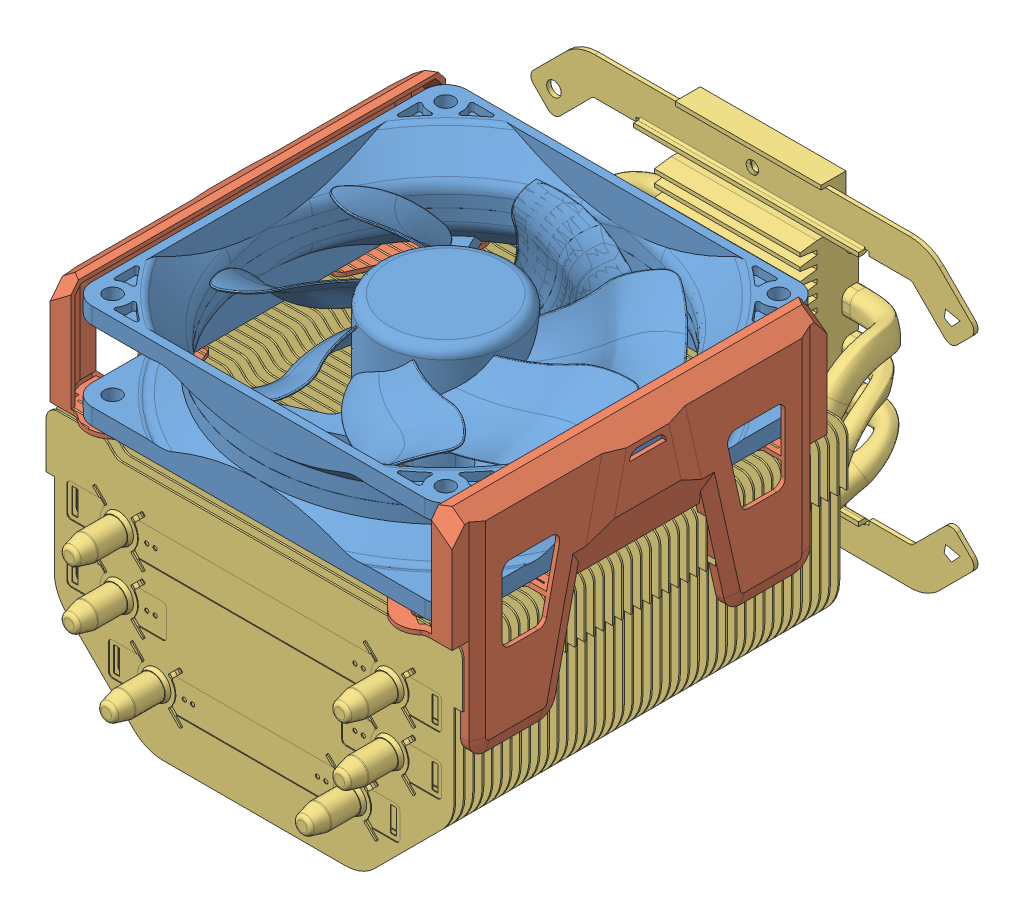
SolidWorks assembly heatsink, configuration Default. Lengths in mm.
Overall size (108.44 87.6 180.01).
4 component instances, 3 part files, 0 mates.
Components (placement in the parent):
- 7030025_PART_FAN STANDARD 90_MODEL.igs-1: 7030025_PART_FAN STANDARD 90_MODEL.igs [Default] at (0 45 -45) x (1 0 0) z (0 -1 0) size (93.98 180.01 25.07)
- 7030026_PART_HEATSINK ADAPTOR 90_MODEL.igs-1: 7030026_PART_HEATSINK ADAPTOR 90_MODEL.igs [Default] at (95 58.5 47.4641) x (0 0 -1) z (-1 0 0) size (106.39 52.6 26.58)
- 7030026_PART_HEATSINK ADAPTOR 90_MODEL.igs-2: 7030026_PART_HEATSINK ADAPTOR 90_MODEL.igs [Default] at (-7 58.5 -46) x (0 0 1) z (1 0 0) size (106.39 52.6 26.58)
- 7030027_PART_CPU HEATSINK TOWER_MODEL.igs-1: 7030027_PART_CPU HEATSINK TOWER_MODEL.igs [Default] at (94 31.5 -47.65) x (-1 0 0) z (0 0 1) size (108.44 80.01 139.76)
